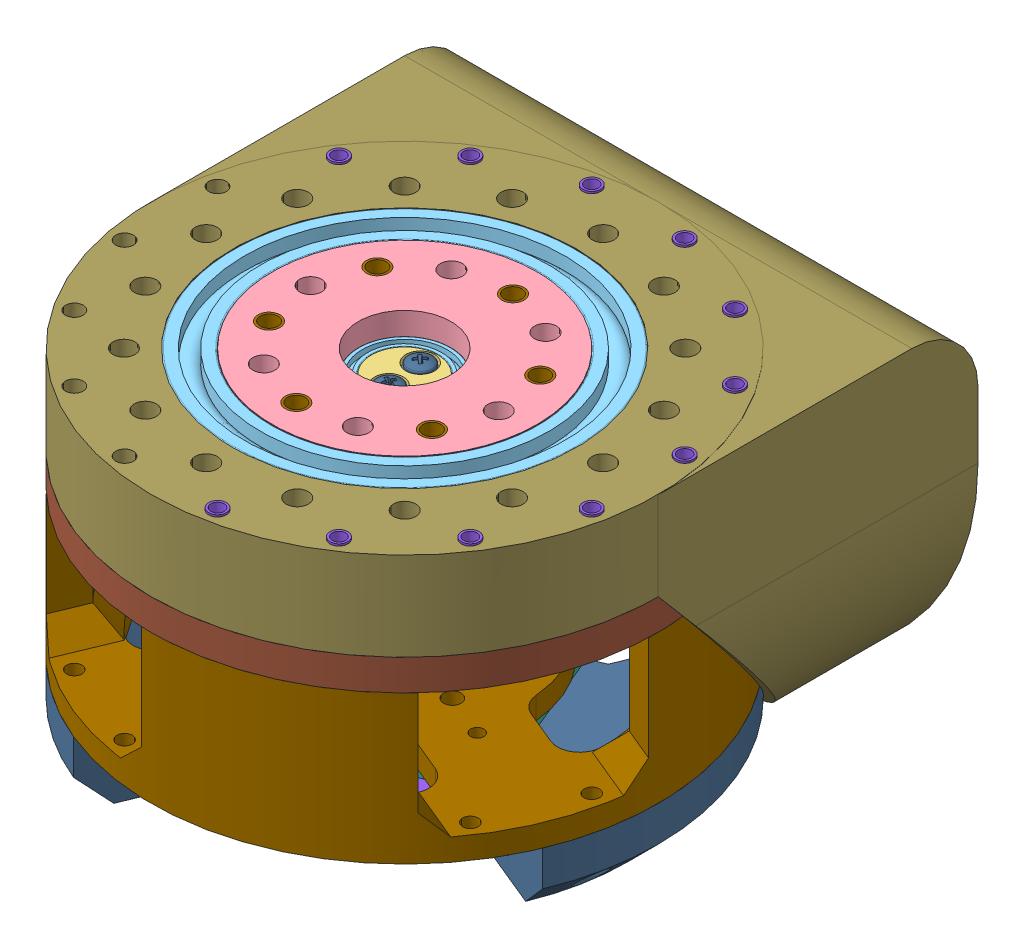
SolidWorks assembly Cycloidal_v3, configuration Default. Lengths in mm.
Overall size (150.25 88 150.25).
358 component instances, 93 part files, 116 mates.
Components (placement in the parent):
- motor-X83008S.stp-1: motor-X83008S.stp [Default] at (43.3116 89.8915 45.5734) x (0.360585 0 0.932726) z (0 -1 0) size (114.7 114.7 37.62) (hidden)
  - base.stp-1: base.stp [Default] at (42.0794 12.0269 46.7342) size (91.6 91.6 15.61)
  - stator.stp-1: stator.stp [Default] at (42.0794 12.0269 33.1342) x (0.08493 -0.996387 0) z (0 0 1) size (83 83 8)
  - coil.stp-1: coil.stp [Default] at (39.5332 41.8984 37.1342) x (0.996387 0.08493 0) z (-0.08493 0.996387 0) size (4.4 10.2 10.5)
  - coil.stp-2: coil.stp [Default] at (34.3848 41.0025 37.1342) x (0.966502 0.256661 0) z (-0.256661 0.966502 0) size (4.4 10.2 10.5)
  - coil.stp-3: coil.stp [Default] at (29.4701 39.2261 37.1342) x (0.90725 0.420593 0) z (-0.420593 0.90725 0) size (4.4 10.2 10.5)
  - coil.stp-4: coil.stp [Default] at (24.9386 36.6233 37.1342) x (0.820431 0.571745 0) z (-0.571745 0.820431 0) size (4.4 10.2 10.5)
  - coil.stp-5: coil.stp [Default] at (20.9279 33.2732 37.1342) x (0.708685 0.705525 0) z (-0.705525 0.708685 0) size (4.4 10.2 10.5)
  - coil.stp-6: coil.stp [Default] at (17.5599 29.2775 37.1342) x (0.575405 0.817869 0) z (-0.817869 0.575405 0) size (4.4 10.2 10.5)
  - coil.stp-7: coil.stp [Default] at (14.9368 24.7576 37.1342) x (0.424642 0.905361 0) z (-0.905361 0.424642 0) size (4.4 10.2 10.5)
  - coil.stp-8: coil.stp [Default] at (13.1385 19.8509 37.1342) x (0.260976 0.965345 0) z (-0.965345 0.260976 0) size (4.4 10.2 10.5)
  - coil.stp-9: coil.stp [Default] at (12.2196 14.7066 37.1342) x (0.089381 0.995998 0) z (-0.995998 0.089381 0) size (4.4 10.2 10.5)
  - coil.stp-10: coil.stp [Default] at (12.2079 9.4807 37.1342) x (-0.08493 0.996387 0) z (-0.996387 -0.08493 0) size (4.4 10.2 10.5)
  - coil.stp-11: coil.stp [Default] at (13.1039 4.3323 37.1342) x (-0.256661 0.966502 0) z (-0.966502 -0.256661 0) size (4.4 10.2 10.5)
  - coil.stp-12: coil.stp [Default] at (14.8802 -0.5824 37.1342) x (-0.420593 0.90725 0) z (-0.90725 -0.420593 0) size (4.4 10.2 10.5)
  - coil.stp-13: coil.stp [Default] at (17.483 -5.1139 37.1342) x (-0.571745 0.820431 0) z (-0.820431 -0.571745 0) size (4.4 10.2 10.5)
  - coil.stp-14: coil.stp [Default] at (20.8332 -9.1246 37.1342) x (-0.705525 0.708685 0) z (-0.708685 -0.705525 0) size (4.4 10.2 10.5)
  - coil.stp-15: coil.stp [Default] at (24.8289 -12.4926 37.1342) x (-0.817869 0.575405 0) z (-0.575405 -0.817869 0) size (4.4 10.2 10.5)
  - coil.stp-16: coil.stp [Default] at (29.3487 -15.1157 37.1342) x (-0.905361 0.424642 0) z (-0.424642 -0.905361 0) size (4.4 10.2 10.5)
  - coil.stp-17: coil.stp [Default] at (34.2554 -16.914 37.1342) x (-0.965345 0.260976 0) z (-0.260976 -0.965345 0) size (4.4 10.2 10.5)
  - coil.stp-18: coil.stp [Default] at (39.3998 -17.8329 37.1342) x (-0.995998 0.089381 0) z (-0.089381 -0.995998 0) size (4.4 10.2 10.5)
  - coil.stp-19: coil.stp [Default] at (44.6256 -17.8446 37.1342) x (-0.996387 -0.08493 0) z (0.08493 -0.996387 0) size (4.4 10.2 10.5)
  - coil.stp-20: coil.stp [Default] at (49.7741 -16.9486 37.1342) x (-0.966502 -0.256661 0) z (0.256661 -0.966502 0) size (4.4 10.2 10.5)
  - coil.stp-21: coil.stp [Default] at (54.6887 -15.1723 37.1342) x (-0.90725 -0.420593 0) z (0.420593 -0.90725 0) size (4.4 10.2 10.5)
  - coil.stp-22: coil.stp [Default] at (59.2202 -12.5695 37.1342) x (-0.820431 -0.571745 0) z (0.571745 -0.820431 0) size (4.4 10.2 10.5)
  - coil.stp-23: coil.stp [Default] at (63.2309 -9.2193 37.1342) x (-0.708685 -0.705525 0) z (0.705525 -0.708685 0) size (4.4 10.2 10.5)
  - coil.stp-24: coil.stp [Default] at (66.599 -5.2236 37.1342) x (-0.575405 -0.817869 0) z (0.817869 -0.575405 0) size (4.4 10.2 10.5)
  - coil.stp-25: coil.stp [Default] at (69.222 -0.7038 37.1342) x (-0.424642 -0.905361 0) z (0.905361 -0.424642 0) size (4.4 10.2 10.5)
  - coil.stp-26: coil.stp [Default] at (71.0203 4.2029 37.1342) x (-0.260976 -0.965345 0) z (0.965345 -0.260976 0) size (4.4 10.2 10.5)
  - coil.stp-27: coil.stp [Default] at (71.9392 9.3473 37.1342) x (-0.089381 -0.995998 0) z (0.995998 -0.089381 0) size (4.4 10.2 10.5)
  - coil.stp-28: coil.stp [Default] at (71.9509 14.5731 37.1342) x (0.08493 -0.996387 0) z (0.996387 0.08493 0) size (4.4 10.2 10.5)
  - coil.stp-29: coil.stp [Default] at (71.055 19.7216 37.1342) x (0.256661 -0.966502 0) z (0.966502 0.256661 0) size (4.4 10.2 10.5)
  - coil.stp-30: coil.stp [Default] at (69.2786 24.6362 37.1342) x (0.420593 -0.90725 0) z (0.90725 0.420593 0) size (4.4 10.2 10.5)
  - coil.stp-31: coil.stp [Default] at (66.6758 29.1677 37.1342) x (0.571745 -0.820431 0) z (0.820431 0.571745 0) size (4.4 10.2 10.5)
  - coil.stp-32: coil.stp [Default] at (63.3257 33.1785 37.1342) x (0.705525 -0.708685 0) z (0.708685 0.705525 0) size (4.4 10.2 10.5)
  - coil.stp-33: coil.stp [Default] at (59.33 36.5465 37.1342) x (0.817869 -0.575405 0) z (0.575405 0.817869 0) size (4.4 10.2 10.5)
  - coil.stp-34: coil.stp [Default] at (54.8101 39.1695 37.1342) x (0.905361 -0.424642 0) z (0.424642 0.905361 0) size (4.4 10.2 10.5)
  - coil.stp-35: coil.stp [Default] at (49.9034 40.9678 37.1342) x (0.965345 -0.260976 0) z (0.260976 0.965345 0) size (4.4 10.2 10.5)
  - coil.stp-36: coil.stp [Default] at (44.759 41.8868 37.1342) x (0.995998 -0.089381 0) z (0.089381 0.995998 0) size (4.4 10.2 10.5)
  - rotor.stp-1: rotor.stp [Default] at (42.0794 12.0269 42.1342) x (-0.293442 0.955977 0) z (0 0 -1) size (91.8 91.8 12)
  - outrunner.stp-1: outrunner.stp [Default] at (42.0794 12.0269 30.1342) x (-0.254711 0.967017 0) z (-0.967017 -0.254711 0) size (91.8 17.01 91.8)
  - screw-mount.stp-1: screw-mount.stp [Default] at (38.1314 27.0157 27.1342) x (1 0 0) z (0 0 -1) size (7 7 6.5)
  - screw-mount.stp-2: screw-mount.stp [Default] at (27.0906 8.0789 27.1342) x (1 0 0) z (0 0 -1) size (7 7 6.5)
  - screw-mount.stp-3: screw-mount.stp [Default] at (57.0682 15.9749 27.1342) x (1 0 0) z (0 0 -1) size (7 7 6.5)
  - screw-mount.stp-4: screw-mount.stp [Default] at (46.0274 -2.9618 27.1342) x (1 0 0) z (0 0 -1) size (7 7 6.5)
  - 6702ZZ-bearing-15x21x4.stp-1: 6702ZZ-bearing-15x21x4.stp [Default] at (42.0794 12.0269 43.7342) x (1 0 0) z (0 -1 0) size (21 4 21)
  - 6702ZZ-bearing-15x21x4.stp-2: 6702ZZ-bearing-15x21x4.stp [Default] at (42.0794 12.0269 35.1342) x (1 0 0) z (0 1 0) size (21 4 21)
  - shaft.stp-1: shaft.stp [Default] at (42.0794 12.0269 20.1342) size (16 16 31.6)
  - fix-screw.stp-1: fix-screw.stp [Default] at (42.0794 12.0269 51.7342) x (1 0 0) z (0 0 -1) size (19.67 18.96 12.02)
- Base_Plate-1: Base_Plate [Default] at (47.267 69.7573 89.1587) x (-0.111117 0 -0.993807) z (0.993807 0 -0.111117) size (40 7 40)
- Eccentric_Shaft-1: Eccentric_Shaft [Default] at (56.4156 70.4165 102.314) x (-0.993807 0 0.111117) z (-0.111117 0 -0.993807) size (20 15 17)
  - Eccentric_Shaft_bot-1: Eccentric_Shaft_bot [Default] at (7.6302 6.3409 14.0904) size (17 5 17)
  - Eccentric_Shaft_bot-2: Eccentric_Shaft_bot [Default] at (7.6302 11.3409 14.0904) x (-1 0 0) z (0 0 -1) size (17 5 17)
  - Eccentric_Shaft_top-1: Eccentric_Shaft_top [Default] at (7.6302 16.3409 14.0904) x (-1 0 0) z (0 0 -1) size (17 5 17)
- Output_Shaft-1: Output_Shaft [Default] at (47.267 86.8173 89.1587) x (-0.997523 0 -0.070342) z (0.070342 0 -0.997523) size (60 10 60)
- radial ball bearing_68_iso-39: radial ball bearing_68_iso [ISO 15 RBB - 1860 - 32,SI,NC,32_68] at (47.267 91.8173 89.1587) x (0 1 0) z (0.105786 0 0.994389) size (10 78 78)
- radial ball bearing_68_iso-40: radial ball bearing_68_iso [ISO 15 RBB - 1840 - 32,SI,NC,32_68] at (47.267 73.2573 89.1587) x (0 1 0) z (-0.019534 0 0.999809) size (7 52 52)
- m13_bearing-31: m13_bearing [Default] at (-10.7414 95.4081 67.0593) x (0.227678 0 0.973736) z (0.973736 0 -0.227678) size (13 16 13)
  - m6-1: m6 [Default] at (8.4921 2.5508 14.8914) size (6 16 6)
  - radial ball bearing_68_iso-1: radial ball bearing_68_iso [ISO 15 RBB - 286 - 10,SI,NC,10_68] at (8.4921 16.0508 14.8914) x (0 1 0) z (0 0 1) size (5 13 13)
  - radial ball bearing_68_iso-2: radial ball bearing_68_iso [ISO 15 RBB - 286 - 10,SI,NC,10_68] at (8.4921 11.0508 14.8914) x (0 1 0) z (0 0 1) size (5 13 13)
- m13_bearing-32: m13_bearing [Default] at (-14.1668 95.4081 84.2801) x (0.227678 0 0.973736) z (0.973736 0 -0.227678) size (13 16 13)
  - m6-1: m6 [Default] at (8.4921 2.5508 14.8914) size (6 16 6)
  - radial ball bearing_68_iso-1: radial ball bearing_68_iso [ISO 15 RBB - 286 - 10,SI,NC,10_68] at (8.4921 16.0508 14.8914) x (0 1 0) z (0 0 1) size (5 13 13)
  - radial ball bearing_68_iso-2: radial ball bearing_68_iso [ISO 15 RBB - 286 - 10,SI,NC,10_68] at (8.4921 11.0508 14.8914) x (0 1 0) z (0 0 1) size (5 13 13)
- m13_bearing-34: m13_bearing [Default] at (13.6125 95.5581 125.8547) x (0.227678 0 0.973736) z (0.973736 0 -0.227678) size (13 16 13)
  - m6-1: m6 [Default] at (8.4921 2.5508 14.8914) size (6 16 6)
  - radial ball bearing_68_iso-1: radial ball bearing_68_iso [ISO 15 RBB - 286 - 10,SI,NC,10_68] at (8.4921 16.0508 14.8914) x (0 1 0) z (0 0 1) size (5 13 13)
  - radial ball bearing_68_iso-2: radial ball bearing_68_iso [ISO 15 RBB - 286 - 10,SI,NC,10_68] at (8.4921 11.0508 14.8914) x (0 1 0) z (0 0 1) size (5 13 13)
- m13_bearing-35: m13_bearing [Default] at (-0.9866 95.4081 116.0999) x (0.227678 0 0.973736) z (0.973736 0 -0.227678) size (13 16 13)
  - m6-1: m6 [Default] at (8.4921 2.5508 14.8914) size (6 16 6)
  - radial ball bearing_68_iso-1: radial ball bearing_68_iso [ISO 15 RBB - 286 - 10,SI,NC,10_68] at (8.4921 16.0508 14.8914) x (0 1 0) z (0 0 1) size (5 13 13)
  - radial ball bearing_68_iso-2: radial ball bearing_68_iso [ISO 15 RBB - 286 - 10,SI,NC,10_68] at (8.4921 11.0508 14.8914) x (0 1 0) z (0 0 1) size (5 13 13)
- m13_bearing-36: m13_bearing [Default] at (-10.7414 95.5581 101.5009) x (0.227678 0 0.973736) z (0.973736 0 -0.227678) size (13 16 13)
  - m6-1: m6 [Default] at (8.4921 2.5508 14.8914) size (6 16 6)
  - radial ball bearing_68_iso-1: radial ball bearing_68_iso [ISO 15 RBB - 286 - 10,SI,NC,10_68] at (8.4921 16.0508 14.8914) x (0 1 0) z (0 0 1) size (5 13 13)
  - radial ball bearing_68_iso-2: radial ball bearing_68_iso [ISO 15 RBB - 286 - 10,SI,NC,10_68] at (8.4921 11.0508 14.8914) x (0 1 0) z (0 0 1) size (5 13 13)
- m13_bearing-1: m13_bearing [Default] at (-0.8801 95.4081 62.5627) x (0.736525 0 0.676411) z (0.676411 0 -0.736525) size (13 16 13)
  - m6-1: m6 [Default] at (8.4921 2.5508 14.8914) size (6 16 6)
  - radial ball bearing_68_iso-1: radial ball bearing_68_iso [ISO 15 RBB - 286 - 10,SI,NC,10_68] at (8.4921 16.0508 14.8914) x (0 1 0) z (0 0 1) size (5 13 13)
  - radial ball bearing_68_iso-2: radial ball bearing_68_iso [ISO 15 RBB - 286 - 10,SI,NC,10_68] at (8.4921 11.0508 14.8914) x (0 1 0) z (0 0 1) size (5 13 13)
- m13_bearing-2: m13_bearing [Default] at (48.6831 95.4081 124.0939) x (0.120271 0 0.992741) z (0.992741 0 -0.120271) size (13 16 13)
  - m6-1: m6 [Default] at (8.4921 2.5508 14.8914) size (6 16 6)
  - radial ball bearing_68_iso-1: radial ball bearing_68_iso [ISO 15 RBB - 286 - 10,SI,NC,10_68] at (8.4921 16.0508 14.8914) x (0 1 0) z (0 0 1) size (5 13 13)
  - radial ball bearing_68_iso-2: radial ball bearing_68_iso [ISO 15 RBB - 286 - 10,SI,NC,10_68] at (8.4921 11.0508 14.8914) x (0 1 0) z (0 0 1) size (5 13 13)
- m13_bearing-3: m13_bearing [Default] at (32.7832 95.4081 34.9886) x (-0.046141 0 0.998935) z (0.998935 0 0.046141) size (13 16 13)
  - m6-1: m6 [Default] at (8.4921 2.5508 14.8914) size (6 16 6)
  - radial ball bearing_68_iso-1: radial ball bearing_68_iso [ISO 15 RBB - 286 - 10,SI,NC,10_68] at (8.4921 16.0508 14.8914) x (0 1 0) z (0 0 1) size (5 13 13)
  - radial ball bearing_68_iso-2: radial ball bearing_68_iso [ISO 15 RBB - 286 - 10,SI,NC,10_68] at (8.4921 11.0508 14.8914) x (0 1 0) z (0 0 1) size (5 13 13)
- m13_bearing-4: m13_bearing [Default] at (77.6928 95.3081 80.133) x (-0.036208 0 0.999344) z (0.999344 0 0.036208) size (13 16 13)
  - m6-1: m6 [Default] at (8.4921 2.5508 14.8914) size (6 16 6)
  - radial ball bearing_68_iso-1: radial ball bearing_68_iso [ISO 15 RBB - 286 - 10,SI,NC,10_68] at (8.4921 16.0508 14.8914) x (0 1 0) z (0 0 1) size (5 13 13)
  - radial ball bearing_68_iso-2: radial ball bearing_68_iso [ISO 15 RBB - 286 - 10,SI,NC,10_68] at (8.4921 11.0508 14.8914) x (0 1 0) z (0 0 1) size (5 13 13)
- m13_bearing-5: m13_bearing [Default] at (73.474 95.4081 98.7828) x (0.059133 0 0.99825) z (0.99825 0 -0.059133) size (13 16 13)
  - m6-1: m6 [Default] at (8.4921 2.5508 14.8914) size (6 16 6)
  - radial ball bearing_68_iso-1: radial ball bearing_68_iso [ISO 15 RBB - 286 - 10,SI,NC,10_68] at (8.4921 16.0508 14.8914) x (0 1 0) z (0 0 1) size (5 13 13)
  - radial ball bearing_68_iso-2: radial ball bearing_68_iso [ISO 15 RBB - 286 - 10,SI,NC,10_68] at (8.4921 11.0508 14.8914) x (0 1 0) z (0 0 1) size (5 13 13)
- m13_bearing-6: m13_bearing [Default] at (12.9248 95.4081 46.7315) x (0.451561 0 0.89224) z (0.89224 0 -0.451561) size (13 16 13)
  - m6-1: m6 [Default] at (8.4921 2.5508 14.8914) size (6 16 6)
  - radial ball bearing_68_iso-1: radial ball bearing_68_iso [ISO 15 RBB - 286 - 10,SI,NC,10_68] at (8.4921 16.0508 14.8914) x (0 1 0) z (0 0 1) size (5 13 13)
  - radial ball bearing_68_iso-2: radial ball bearing_68_iso [ISO 15 RBB - 286 - 10,SI,NC,10_68] at (8.4921 11.0508 14.8914) x (0 1 0) z (0 0 1) size (5 13 13)
- m13_bearing-7: m13_bearing [Default] at (56.6452 95.4081 32.3406) x (-0.545813 0 0.837907) z (0.837907 0 0.545813) size (13 16 13)
  - m6-1: m6 [Default] at (8.4921 2.5508 14.8914) size (6 16 6)
  - radial ball bearing_68_iso-1: radial ball bearing_68_iso [ISO 15 RBB - 286 - 10,SI,NC,10_68] at (8.4921 16.0508 14.8914) x (0 1 0) z (0 0 1) size (5 13 13)
  - radial ball bearing_68_iso-2: radial ball bearing_68_iso [ISO 15 RBB - 286 - 10,SI,NC,10_68] at (8.4921 11.0508 14.8914) x (0 1 0) z (0 0 1) size (5 13 13)
- m13_bearing-8: m13_bearing [Default] at (63.0373 95.4081 51.3153) x (0.158553 0 0.98735) z (0.98735 0 -0.158553) size (13 16 13)
  - m6-1: m6 [Default] at (8.4921 2.5508 14.8914) size (6 16 6)
  - radial ball bearing_68_iso-1: radial ball bearing_68_iso [ISO 15 RBB - 286 - 10,SI,NC,10_68] at (8.4921 16.0508 14.8914) x (0 1 0) z (0 0 1) size (5 13 13)
  - radial ball bearing_68_iso-2: radial ball bearing_68_iso [ISO 15 RBB - 286 - 10,SI,NC,10_68] at (8.4921 11.0508 14.8914) x (0 1 0) z (0 0 1) size (5 13 13)
- m13_bearing-9: m13_bearing [Default] at (83.8577 95.4081 55.5358) x (-0.687134 0 0.72653) z (0.72653 0 0.687134) size (13 16 13)
  - m6-1: m6 [Default] at (8.4921 2.5508 14.8914) size (6 16 6)
  - radial ball bearing_68_iso-1: radial ball bearing_68_iso [ISO 15 RBB - 286 - 10,SI,NC,10_68] at (8.4921 16.0508 14.8914) x (0 1 0) z (0 0 1) size (5 13 13)
  - radial ball bearing_68_iso-2: radial ball bearing_68_iso [ISO 15 RBB - 286 - 10,SI,NC,10_68] at (8.4921 11.0508 14.8914) x (0 1 0) z (0 0 1) size (5 13 13)
- m13_bearing-11: m13_bearing [Default] at (30.1977 95.4081 135.7424) x (0.57351 0 0.819198) z (0.819198 0 -0.57351) size (13 16 13)
  - m6-1: m6 [Default] at (8.4921 2.5508 14.8914) size (6 16 6)
  - radial ball bearing_68_iso-1: radial ball bearing_68_iso [ISO 15 RBB - 286 - 10,SI,NC,10_68] at (8.4921 16.0508 14.8914) x (0 1 0) z (0 0 1) size (5 13 13)
  - radial ball bearing_68_iso-2: radial ball bearing_68_iso [ISO 15 RBB - 286 - 10,SI,NC,10_68] at (8.4921 11.0508 14.8914) x (0 1 0) z (0 0 1) size (5 13 13)
- m13_bearing-12: m13_bearing [Default] at (62.8861 95.4081 115.3744) x (0.184178 0 0.982893) z (0.982893 0 -0.184178) size (13 16 13)
  - m6-1: m6 [Default] at (8.4921 2.5508 14.8914) size (6 16 6)
  - radial ball bearing_68_iso-1: radial ball bearing_68_iso [ISO 15 RBB - 286 - 10,SI,NC,10_68] at (8.4921 16.0508 14.8914) x (0 1 0) z (0 0 1) size (5 13 13)
  - radial ball bearing_68_iso-2: radial ball bearing_68_iso [ISO 15 RBB - 286 - 10,SI,NC,10_68] at (8.4921 11.0508 14.8914) x (0 1 0) z (0 0 1) size (5 13 13)
- socket button head screw_iso-2: socket button head screw_iso [ISO 7380 - M4 x 12 - 12N] at (47.267 67.4573 134.1587) x (0 1 0) z (-0.724148 0 0.689645) size (14.2 7.6 7.6)
- socket button head screw_iso-3: socket button head screw_iso [ISO 7380 - M4 x 12 - 12N] at (15.4472 67.4573 57.3389) x (0 1 0) z (-0.724148 0 0.689645) size (14.2 7.6 7.6)
- socket button head screw_iso-4: socket button head screw_iso [ISO 7380 - M4 x 12 - 12N] at (30.0462 67.4573 47.5841) x (0 1 0) z (-0.724148 0 0.689645) size (14.2 7.6 7.6)
- socket button head screw_iso-5: socket button head screw_iso [ISO 7380 - M4 x 12 - 12N] at (47.267 67.4573 44.1587) x (0 1 0) z (-0.724148 0 0.689645) size (14.2 7.6 7.6)
- socket button head screw_iso-6: socket button head screw_iso [ISO 7380 - M4 x 12 - 12N] at (64.4877 67.4573 47.5841) x (0 1 0) z (-0.724148 0 0.689645) size (14.2 7.6 7.6)
- socket button head screw_iso-8: socket button head screw_iso [ISO 7380 - M4 x 12 - 12N] at (88.8416 67.4573 71.9379) x (0 1 0) z (-0.724148 0 0.689645) size (14.2 7.6 7.6)
- socket button head screw_iso-9: socket button head screw_iso [ISO 7380 - M4 x 12 - 12N] at (92.267 67.4573 89.1587) x (0 1 0) z (-0.724148 0 0.689645) size (14.2 7.6 7.6)
- socket button head screw_iso-10: socket button head screw_iso [ISO 7380 - M4 x 12 - 12N] at (88.8416 67.4573 106.3794) x (0 1 0) z (-0.724148 0 0.689645) size (14.2 7.6 7.6)
- socket button head screw_iso-11: socket button head screw_iso [ISO 7380 - M4 x 12 - 12N] at (79.0868 67.4573 120.9785) x (0 1 0) z (-0.724148 0 0.689645) size (14.2 7.6 7.6)
- M3x4x4.2_brass_insert-2: M3x4x4.2_brass_insert [Default] at (2.3676 97.2573 59.1579) x (-0.680278 0 -0.732954) z (-0.732954 0 0.680278) size (4 4 4)
- M3x4x4.2_brass_insert-3: M3x4x4.2_brass_insert [Default] at (17.2662 97.2573 44.2593) x (-0.509546 0 -0.860444) z (-0.860444 0 0.509546) size (4 4 4)
- M3x4x4.2_brass_insert-6: M3x4x4.2_brass_insert [Default] at (77.2678 97.2573 44.2593) x (-0.680278 0 -0.732954) z (-0.732954 0 0.680278) size (4 4 4)
- M3x4x4.2_brass_insert-8: M3x4x4.2_brass_insert [Default] at (100.2294 93.2573 78.6238) x (-0.970393 0 0.241533) z (-0.241533 0 -0.970393) size (4 4 4)
- M3x4x4.2_brass_insert-14: M3x4x4.2_brass_insert [Default] at (36.7321 97.2573 36.1963) x (0.509546 0 0.860444) z (0.860444 0 -0.509546) size (4 4 4)
- M3x4x4.2_brass_insert-15: M3x4x4.2_brass_insert [Default] at (57.8019 93.2573 36.1963) x (0.897191 0 -0.441644) z (0.441644 0 0.897191) size (4 4 4)
- M3x4x4.2_brass_insert-16: M3x4x4.2_brass_insert [Default] at (92.1663 97.2573 59.1579) x (-0.680278 0 -0.732954) z (-0.732954 0 0.680278) size (4 4 4)
- M3x4x4.2_brass_insert-17: M3x4x4.2_brass_insert [Default] at (100.2294 97.2573 99.6935) x (0.680278 0 0.732954) z (0.732954 0 -0.680278) size (4 4 4)
- M3x4x4.2_brass_insert-19: M3x4x4.2_brass_insert [Default] at (92.1663 97.2573 119.1595) x (0.680278 0 0.732954) z (0.732954 0 -0.680278) size (4 4 4)
- M3x4x4.2_brass_insert-20: M3x4x4.2_brass_insert [Default] at (77.2678 97.2573 134.058) x (0.680278 0 0.732954) z (0.732954 0 -0.680278) size (4 4 4)
- M3x4x4.2_brass_insert-21: M3x4x4.2_brass_insert [Default] at (57.8019 97.2573 142.1211) x (0.680278 0 0.732954) z (0.732954 0 -0.680278) size (4 4 4)
- M4x6x5.5_brass_insert-47: M4x6x5.5_brass_insert [Default] at (5.6924 92.8573 71.9379) x (0.474598 0 0.880203) z (0 1 0) size (5 5 6)
- M4x6x5.5_brass_insert-48: M4x6x5.5_brass_insert [Default] at (2.267 92.8573 89.1587) x (0.260051 0 0.965595) z (0 1 0) size (5 5 6)
- M4x6x5.5_brass_insert-49: M4x6x5.5_brass_insert [Default] at (5.6924 87.0073 106.3794) x (-0.745833 0 0.666133) z (0 -1 0) size (5 5 6)
- M4x6x5.5_brass_insert-50: M4x6x5.5_brass_insert [Default] at (15.4472 86.8573 120.9785) x (-0.745833 0 0.666133) z (0 -1 0) size (5 5 6)
- M4x6x5.5_brass_insert-51: M4x6x5.5_brass_insert [Default] at (30.0462 87.0073 130.7332) x (0.260051 0 -0.965595) z (0 -1 0) size (5 5 6)
- M4x6x5.5_brass_insert-1: M4x6x5.5_brass_insert [Default] at (37.1966 86.633 68.4805) x (-0.745833 0 0.666133) z (0 -1 0) size (5 5 6)
- M4x6x5.5_brass_insert-4: M4x6x5.5_brass_insert [Default] at (70.21 92.633 90.7765) x (0.260051 0 0.965595) z (0 1 0) size (5 5 6)
- M4x6x5.5_brass_insert-5: M4x6x5.5_brass_insert [Default] at (57.3374 92.633 109.8369) x (0.260051 0 0.965595) z (0 1 0) size (5 5 6)
- M4x6x5.5_brass_insert-6: M4x6x5.5_brass_insert [Default] at (34.3944 92.633 108.219) x (0.252509 0 0.967595) z (0 1 0) size (5 5 6)
- M4x6x5.5_brass_insert-7: M4x6x5.5_brass_insert [Default] at (24.324 92.633 87.5408) x (0.175665 0 0.98445) z (0 1 0) size (5 5 6)
- M4x6x5.5_brass_insert-8: M4x6x5.5_brass_insert [Default] at (48.8849 96.8173 66.2156) x (0.294696 0 0.955591) z (0 1 0) size (5 5 6)
- M4x6x5.5_brass_insert-9: M4x6x5.5_brass_insert [Default] at (28.2067 96.8173 76.286) x (0.260051 0 0.965595) z (0 1 0) size (5 5 6)
- M4x6x5.5_brass_insert-10: M4x6x5.5_brass_insert [Default] at (26.5888 96.8173 99.2291) x (0.009651 0 0.999953) z (0 1 0) size (5 5 6)
- M4x6x5.5_brass_insert-11: M4x6x5.5_brass_insert [Default] at (45.6491 96.8173 112.1017) x (0.260051 0 0.965595) z (0 1 0) size (5 5 6)
- M4x6x5.5_brass_insert-13: M4x6x5.5_brass_insert [Default] at (66.3273 96.8173 102.0313) x (0.260051 0 0.965595) z (0 1 0) size (5 5 6)
- M4x6x5.5_brass_insert-14: M4x6x5.5_brass_insert [Default] at (67.9452 96.8173 79.0883) x (0.260051 0 0.965595) z (0 1 0) size (5 5 6)
- M4x6x5.5_brass_insert-15: M4x6x5.5_brass_insert [Default] at (60.1396 92.633 70.0984) x (0.151918 0 0.988393) z (0 1 0) size (5 5 6)
- M4x6x5.5_brass_insert-20: M4x6x5.5_brass_insert [Default] at (64.4877 86.8573 130.7332) x (-0.745833 0 0.666133) z (0 -1 0) size (5 5 6)
- M4x6x5.5_brass_insert-21: M4x6x5.5_brass_insert [Default] at (47.267 86.8573 134.1587) x (-0.745833 0 0.666133) z (0 -1 0) size (5 5 6)
- M4x6x5.5_brass_insert-22: M4x6x5.5_brass_insert [Default] at (15.4472 86.8573 57.3389) x (0.623293 0 0.781988) z (0 -1 0) size (5 5 6)
- M4x6x5.5_brass_insert-23: M4x6x5.5_brass_insert [Default] at (30.0462 86.8573 47.5841) x (0.623293 0 0.781988) z (0 -1 0) size (5 5 6)
- M4x6x5.5_brass_insert-24: M4x6x5.5_brass_insert [Default] at (79.0868 86.8573 120.9785) x (0.541965 0 0.840401) z (0 -1 0) size (5 5 6)
- M4x6x5.5_brass_insert-25: M4x6x5.5_brass_insert [Default] at (88.8416 86.8573 106.3794) x (-0.745833 0 0.666133) z (0 -1 0) size (5 5 6)
- M4x6x5.5_brass_insert-26: M4x6x5.5_brass_insert [Default] at (92.267 86.8573 89.1587) x (-0.745833 0 0.666133) z (0 -1 0) size (5 5 6)
- M4x6x5.5_brass_insert-27: M4x6x5.5_brass_insert [Default] at (88.8416 86.8573 71.9379) x (-0.745833 0 0.666133) z (0 -1 0) size (5 5 6)
- M4x6x5.5_brass_insert-28: M4x6x5.5_brass_insert [Default] at (79.0868 92.8573 57.3389) x (0.260051 0 0.965595) z (0 1 0) size (5 5 6)
- M4x6x5.5_brass_insert-29: M4x6x5.5_brass_insert [Default] at (64.4877 86.8573 47.5841) x (-0.142939 0 0.989731) z (0 -1 0) size (5 5 6)
- M4x6x5.5_brass_insert-31: M4x6x5.5_brass_insert [Default] at (47.267 86.8573 44.1587) x (-0.220341 0 0.975423) z (0 -1 0) size (5 5 6)
- pan cross head_am-1: pan cross head_am [B18.6.7M - M3 x 0.5 x 20 Type I Cross Recessed PHMS --20N] at (46.8225 92.6573 85.1834) x (0 -1 0) z (0.748822 0 0.662771) size (22.37 5.6 5.6)
- pan cross head_am-3: pan cross head_am [B18.6.7M - M3 x 0.5 x 20 Type I Cross Recessed PHMS --20N] at (47.7115 92.6573 93.1339) x (0 -1 0) z (0.940321 0 0.340288) size (22.37 5.6 5.6)
- M3x4x4.2_brass_insert-22: M3x4x4.2_brass_insert [Default] at (46.8225 69.7573 85.1834) x (0.984578 0 -0.174944) z (0.174944 0 0.984578) size (4 4 4)
- M3x4x4.2_brass_insert-23: M3x4x4.2_brass_insert [Default] at (47.7115 69.7573 93.1339) x (0.984609 0 -0.174769) z (0.174769 0 0.984609) size (4 4 4)
- pan cross head_am-4: pan cross head_am [B18.6.7M - M3 x 0.5 x 10 Type I Cross Recessed PHMS --10N] at (48.9893 77.6573 104.5627) x (0 -1 0) z (0 0 1) size (12.37 5.6 5.6)
- pan cross head_am-5: pan cross head_am [B18.6.7M - M3 x 0.5 x 10 Type I Cross Recessed PHMS --10N] at (45.5447 77.6573 73.7547) x (0 -1 0) z (0 0 1) size (12.37 5.6 5.6)
- pan cross head_am-6: pan cross head_am [B18.6.7M - M3 x 0.5 x 10 Type I Cross Recessed PHMS --10N] at (62.671 77.6573 87.4364) x (0 -1 0) z (0 0 1) size (12.37 5.6 5.6)
- pan cross head_am-7: pan cross head_am [B18.6.7M - M3 x 0.5 x 10 Type I Cross Recessed PHMS --10N] at (31.863 77.6573 90.881) x (0 -1 0) z (0 0 1) size (12.37 5.6 5.6)
- radial ball bearing_68_iso-44: radial ball bearing_68_iso [ISO 15 RBB - 1715 - 26,SI,NC,26_68] at (45.7763 84.7573 89.3253) x (0 1 0) z (-0.714953 0 -0.699173) size (4 21 21)
- radial ball bearing_68_iso-45: radial ball bearing_68_iso [ISO 15 RBB - 1715 - 26,SI,NC,26_68] at (47.267 89.7573 89.1587) x (0 1 0) z (0.999483 0 -0.032163) size (4 21 21)
- radial ball bearing_68_iso-46: radial ball bearing_68_iso [ISO 15 RBB - 1715 - 26,SI,NC,26_68] at (48.7577 79.7573 88.992) x (0 1 0) z (0.000177 0 1) size (4 21 21)
- socket button head screw_iso-37: socket button head screw_iso [ISO 7380 - M4 x 12 - 12N] at (79.0868 67.4573 57.3389) x (0 1 0) z (-0.709975 0 0.704227) size (14.2 7.6 7.6)
- socket button head screw_iso-38: socket button head screw_iso [ISO 7380 - M4 x 12 - 12N] at (64.4877 67.4573 130.7332) x (0 1 0) z (-0.724148 0 0.689645) size (14.2 7.6 7.6)
- foc-motor-controller.step-1: foc-motor-controller.step [Default] at (47.267 33.7573 89.1587) x (-0.382683 0 -0.92388) z (0 -1 0) size (57.23 50 8.13)
  - RTA0040B.step-1: RTA0040B.step [Default] at (12.5014 -1.6986 1.595) x (-0.707107 -0.707107 0) z (0 0 1) size (6 6 1)
    - FRAME.step-1: FRAME.step [Default] x (1 0 0) z (0 -1 0) size (6 0.2 6)
      - SOLID.step-1: SOLID.step [Default] at origin size (0.4 0.2 0.22)
      - SOLID-0.step-1: SOLID-0.step [Default] at origin size (0.4 0.2 0.22)
      - SOLID-1.step-1: SOLID-1.step [Default] at origin size (0.4 0.2 0.22)
      - SOLID-2.step-1: SOLID-2.step [Default] at origin size (0.4 0.2 0.22)
      - SOLID-3.step-1: SOLID-3.step [Default] at origin size (0.4 0.2 0.22)
      - SOLID-4.step-1: SOLID-4.step [Default] at origin size (0.4 0.2 0.22)
      - SOLID-5.step-1: SOLID-5.step [Default] at origin size (0.4 0.2 0.22)
      - SOLID-6.step-1: SOLID-6.step [Default] at origin size (0.4 0.2 0.22)
      - SOLID-7.step-1: SOLID-7.step [Default] at origin size (0.4 0.2 0.22)
      - SOLID-8.step-1: SOLID-8.step [Default] at origin size (0.4 0.2 0.22)
      - SOLID-9.step-1: SOLID-9.step [Default] at origin size (0.22 0.2 0.4)
      - SOLID-10.step-1: SOLID-10.step [Default] at origin size (0.22 0.2 0.4)
      - SOLID-11.step-1: SOLID-11.step [Default] at origin size (0.22 0.2 0.4)
      - SOLID-12.step-1: SOLID-12.step [Default] at origin size (0.22 0.2 0.4)
      - SOLID-13.step-1: SOLID-13.step [Default] at origin size (0.22 0.2 0.4)
      - SOLID-14.step-1: SOLID-14.step [Default] at origin size (0.22 0.2 0.4)
      - SOLID-15.step-1: SOLID-15.step [Default] at origin size (0.22 0.2 0.4)
      - SOLID-16.step-1: SOLID-16.step [Default] at origin size (0.22 0.2 0.4)
      - SOLID-17.step-1: SOLID-17.step [Default] at origin size (4.15 0.2 4.15)
      - SOLID-18.step-1: SOLID-18.step [Default] at origin size (0.28 0.1 0.28)
      - SOLID-19.step-1: SOLID-19.step [Default] at origin size (0.28 0.1 0.28)
      - SOLID-20.step-1: SOLID-20.step [Default] at origin size (0.28 0.1 0.28)
      - SOLID-21.step-1: SOLID-21.step [Default] at origin size (0.28 0.1 0.28)
      - SOLID-22.step-1: SOLID-22.step [Default] at origin size (0.4 0.2 0.22)
      - SOLID-23.step-1: SOLID-23.step [Default] at origin size (0.4 0.2 0.22)
      - SOLID-24.step-1: SOLID-24.step [Default] at origin size (0.4 0.2 0.22)
      - SOLID-25.step-1: SOLID-25.step [Default] at origin size (0.4 0.2 0.22)
      - SOLID-26.step-1: SOLID-26.step [Default] at origin size (0.4 0.2 0.22)
      - SOLID-27.step-1: SOLID-27.step [Default] at origin size (0.4 0.2 0.22)
      - SOLID-28.step-1: SOLID-28.step [Default] at origin size (0.4 0.2 0.22)
      - SOLID-29.step-1: SOLID-29.step [Default] at origin size (0.4 0.2 0.22)
      - SOLID-30.step-1: SOLID-30.step [Default] at origin size (0.4 0.2 0.22)
      - SOLID-31.step-1: SOLID-31.step [Default] at origin size (0.4 0.2 0.22)
      - SOLID-32.step-1: SOLID-32.step [Default] at origin size (0.22 0.2 0.4)
      - SOLID-33.step-1: SOLID-33.step [Default] at origin size (0.22 0.2 0.4)
      - SOLID-34.step-1: SOLID-34.step [Default] at origin size (0.22 0.2 0.4)
      - SOLID-35.step-1: SOLID-35.step [Default] at origin size (0.22 0.2 0.4)
      - SOLID-36.step-1: SOLID-36.step [Default] at origin size (0.22 0.2 0.4)
      - SOLID-37.step-1: SOLID-37.step [Default] at origin size (0.22 0.2 0.4)
      - SOLID-38.step-1: SOLID-38.step [Default] at origin size (0.22 0.2 0.4)
      - SOLID-39.step-1: SOLID-39.step [Default] at origin size (0.22 0.2 0.4)
      - SOLID-40.step-1: SOLID-40.step [Default] at origin size (0.22 0.2 0.4)
      - SOLID-41.step-1: SOLID-41.step [Default] at origin size (0.22 0.2 0.4)
      - SOLID-42.step-1: SOLID-42.step [Default] at origin size (0.22 0.2 0.4)
      - SOLID-43.step-1: SOLID-43.step [Default] at origin size (0.22 0.2 0.4)
    - BODY.step-1: BODY.step [Default] at (0 0 0.025) x (1 0 0) z (0 -1 0) size (6 0.97 6)
  - Resonator_SMD_Murata_CSTxExxV-3Pin_3.0x1.1mm.step-1: Resonator_SMD_Murata_CSTxExxV-3Pin_3.0x1.1mm.step [Default] at (1.8 -7 1.595) x (0 1 0) z (0 0 1) size (3.2 1.35 0.9)
  - C_0603_1608Metric.step-1: C_0603_1608Metric.step [Default] at (6.2 -16.8 1.595) x (0 -1 0) z (0 0 1) size (1.6 0.8 0.8)
  - R_0603_1608Metric.step-1: R_0603_1608Metric.step [Default] at (11.8 -7.375 1.595) x (0 1 0) z (0 0 1) size (1.6 0.8 0.45)
  - R_0603_1608Metric.step-2: R_0603_1608Metric.step [Default] at (13.8 -16.8 1.595) x (0 1 0) z (0 0 1) size (1.6 0.8 0.45)
  - R_0603_1608Metric.step-3: R_0603_1608Metric.step [Default] at (18.1 -5.36 1.595) size (1.6 0.8 0.45)
  - C_0603_1608Metric.step-2: C_0603_1608Metric.step [Default] at (2.6 -0.5 1.595) x (0 -1 0) z (0 0 1) size (1.6 0.8 0.8)
  - R_0603_1608Metric.step-4: R_0603_1608Metric.step [Default] at (14.6 -11.3 1.595) x (0 1 0) z (0 0 1) size (1.6 0.8 0.45)
  - L_APV_ANR4020.step-1: L_APV_ANR4020.step [Default] at (22.3 -13.7 1.595) x (0 -1 0) z (0 0 1) size (4.02 4 2)
  - C_0603_1608Metric.step-3: C_0603_1608Metric.step [Default] at (0.3 -12.6 1.595) x (-1 0 0) z (0 0 1) size (1.6 0.8 0.8)
  - C_1206_3216Metric.step-1: C_1206_3216Metric.step [Default] at (15.7 11 1.595) x (0 1 0) z (0 0 1) size (3.2 1.6 1.6)
  - C_0603_1608Metric.step-4: C_0603_1608Metric.step [Default] at (0.3 -9.6 1.595) size (1.6 0.8 0.8)
  - R_0603_1608Metric.step-5: R_0603_1608Metric.step [Default] at (12.3 -16.8 1.595) x (0 1 0) z (0 0 1) size (1.6 0.8 0.45)
  - C_0603_1608Metric.step-5: C_0603_1608Metric.step [Default] at (-0.3 -16.6 1.595) x (0 1 0) z (0 0 1) size (1.6 0.8 0.8)
  - R_0603_1608Metric.step-6: R_0603_1608Metric.step [Default] at (10.9 4.1 1.595) size (1.6 0.8 0.45)
  - C_1206_3216Metric.step-2: C_1206_3216Metric.step [Default] at (6.3 11 1.595) x (0 1 0) z (0 0 1) size (3.2 1.6 1.6)
  - XT30PW_2_2_-M.G.B.step-1: XT30PW_2_2_-M.G.B.step [Default] at (-20.5 9.5 1.595) x (0 -1 0) z (-1 0 0) size (15.5 7.1 12.53)
  - R_0603_1608Metric.step-7: R_0603_1608Metric.step [Default] at (0.3 -11.1 1.595) size (1.6 0.8 0.45)
  - C_0603_1608Metric.step-6: C_0603_1608Metric.step [Default] at (19 -0.4 1.595) x (-0.707107 -0.707107 0) z (0 0 1) size (1.6 0.8 0.8)
  - C_1206_3216Metric.step-3: C_1206_3216Metric.step [Default] at (13.3 11 1.595) x (0 1 0) z (0 0 1) size (3.2 1.6 1.6)
  - R_0603_1608Metric.step-8: R_0603_1608Metric.step [Default] at (10.2 -7.375 1.595) x (0 -1 0) z (0 0 1) size (1.6 0.8 0.45)
  - JST_GH_SM08B-GHS-TB_1x08-1MP_P1.25mm_Horizontal.step-1: JST_GH_SM08B-GHS-TB_1x08-1MP_P1.25mm_Horizontal.step [Default] at (10 -22 1.595) size (13.25 4.95 4.25)
  - C_1206_3216Metric.step-4: C_1206_3216Metric.step [Default] at (-12.3 11 1.595) x (0 1 0) z (0 0 1) size (3.2 1.6 1.6)
  - JST_GH_SM06B-GHS-TB_1x06-1MP_P1.25mm_Horizontal.step-1: JST_GH_SM06B-GHS-TB_1x06-1MP_P1.25mm_Horizontal.step [Default] at (-4.3 -22 1.595) size (10.75 4.95 4.25)
  - C_0603_1608Metric.step-7: C_0603_1608Metric.step [Default] at (7.3 -4.5 1.595) x (-1 0 0) z (0 0 1) size (1.6 0.8 0.8)
  - R_0603_1608Metric.step-9: R_0603_1608Metric.step [Default] at (18.1 -3.86 1.595) x (-1 0 0) z (0 0 1) size (1.6 0.8 0.45)
  - C_1206_3216Metric.step-5: C_1206_3216Metric.step [Default] at (22.6794 -1.2206 1.595) x (0.707107 -0.707107 0) z (0 0 1) size (3.2 1.6 1.6)
  - R_Array_Convex_4x0402.step-1: R_Array_Convex_4x0402.step [Default] at (6.8 -2.5 1.595) size (1 2 0.35)
  - R_0603_1608Metric.step-10: R_0603_1608Metric.step [Default] at (7.7 -16.8 1.595) x (0 -1 0) z (0 0 1) size (1.6 0.8 0.45)
  - C_1206_3216Metric.step-6: C_1206_3216Metric.step [Default] at (8.7 11 1.595) x (0 1 0) z (0 0 1) size (3.2 1.6 1.6)
  - C_0603_1608Metric.step-8: C_0603_1608Metric.step [Default] at (16.1 -11.3 1.595) x (0 1 0) z (0 0 1) size (1.6 0.8 0.8)
  - SOT-23-5.step-1: SOT-23-5.step [Default] at (-3.1 -16.6 1.595) x (-1 0 0) z (0 0 1) size (2.8 2.9 1.55)
  - C_0603_1608Metric.step-9: C_0603_1608Metric.step [Default] at (17.8 -13.6 1.595) size (1.6 0.8 0.8)
  - R_0603_1608Metric.step-11: R_0603_1608Metric.step [Default] at (-11.5 -20.3875 1.595) x (0 -1 0) z (0 0 1) size (1.6 0.8 0.45)
  - C_0603_1608Metric.step-10: C_0603_1608Metric.step [Default] at (-12.4 2.3 1.595) x (0 1 0) z (0 0 1) size (1.6 0.8 0.8)
  - C_1206_3216Metric.step-7: C_1206_3216Metric.step [Default] at (18 11 1.595) x (0 1 0) z (0 0 1) size (3.2 1.6 1.6)
  - R_0603_1608Metric.step-12: R_0603_1608Metric.step [Default] at (-10.8105 -14.9971 1.595) x (-1 0 0) z (0 0 1) size (1.6 0.8 0.45)
  - C_0603_1608Metric.step-11: C_0603_1608Metric.step [Default] at (-13.8 -9.4 1.595) x (-1 0 0) z (0 0 1) size (1.6 0.8 0.8)
  - R_0603_1608Metric.step-13: R_0603_1608Metric.step [Default] at (-23.15 -14.5 1.595) x (-1 0 0) z (0 0 1) size (1.6 0.8 0.45)
  - C_0603_1608Metric.step-12: C_0603_1608Metric.step [Default] at (1.1 -0.2 1.595) x (0 1 0) z (0 0 1) size (1.6 0.8 0.8)
  - D_0805_2012Metric.step-1: D_0805_2012Metric.step [Default] at (22.9 -9.6 1.595) x (0 1 0) z (0 0 1) size (2 1.27 0.8)
  - C_0603_1608Metric.step-13: C_0603_1608Metric.step [Default] at (-7.8 3.775 1.595) x (0 -1 0) z (0 0 1) size (1.6 0.8 0.8)
  - R_0603_1608Metric.step-14: R_0603_1608Metric.step [Default] at (-6.4 -12.825 1.595) x (0 1 0) z (0 0 1) size (1.6 0.8 0.45)
  - L_0603_1608Metric.step-1: L_0603_1608Metric.step [Default] at (-10.1 3 1.595) size (1.6 0.8 0.8)
  - C_0603_1608Metric.step-14: C_0603_1608Metric.step [Default] at (17.9 0.7 1.595) x (-0.707107 -0.707107 0) z (0 0 1) size (1.6 0.8 0.8)
  - HVSSOP-10.step-1: HVSSOP-10.step [Default] at (18.6 -9.6 1.595) x (0 -1 0) z (-1 0 0) size (4.9 1.1 3)
  - C_0603_1608Metric.step-15: C_0603_1608Metric.step [Default] at (7.9 4.1 1.595) x (-1 0 0) z (0 0 1) size (1.6 0.8 0.8)
  - C_0603_1608Metric.step-16: C_0603_1608Metric.step [Default] at (21.1 -9.6 1.595) x (0 -1 0) z (0 0 1) size (1.6 0.8 0.8)
  - R_0603_1608Metric.step-15: R_0603_1608Metric.step [Default] at (-10.8105 -11.9971 1.595) x (-1 0 0) z (0 0 1) size (1.6 0.8 0.45)
  - R_0603_1608Metric.step-16: R_0603_1608Metric.step [Default] at (-18.2 -17.4 1.595) size (1.6 0.8 0.45)
  - C_1206_3216Metric.step-8: C_1206_3216Metric.step [Default] at (-3 11 1.595) x (0 1 0) z (0 0 1) size (3.2 1.6 1.6)
  - R_0603_1608Metric.step-17: R_0603_1608Metric.step [Default] at (-16.9 -20.4 1.595) x (0 -1 0) z (0 0 1) size (1.6 0.8 0.45)
  - R_0603_1608Metric.step-18: R_0603_1608Metric.step [Default] at (-13.3 -20.3875 1.595) x (0 -1 0) z (0 0 1) size (1.6 0.8 0.45)
  - R_0603_1608Metric.step-19: R_0603_1608Metric.step [Default] at (-15.1 -20.3875 1.595) x (0 -1 0) z (0 0 1) size (1.6 0.8 0.45)
  - C_0603_1608Metric.step-17: C_0603_1608Metric.step [Default] at (15.5 -14.4 1.595) x (0 -1 0) z (0 0 1) size (1.6 0.8 0.8)
  - LED_0603_1608Metric.step-1: LED_0603_1608Metric.step [Default] at (-11.5 -23.3875 1.595) x (0 1 0) z (0 0 1) size (1.6 0.8 1.1)
  - C_0805_2012Metric.step-1: C_0805_2012Metric.step [Default] at (19.95 -17 1.595) size (2 1.25 1.25)
  - D_SMB.step-1: D_SMB.step [Default] at (-16.5 11.208 1.595) x (0 -1 0) z (0 0 1) size (5.3 3.55 2.15)
  - C_1206_3216Metric.step-9: C_1206_3216Metric.step [Default] at (-5.3 11 1.595) x (0 1 0) z (0 0 1) size (3.2 1.6 1.6)
  - XT30PW_2_2_-M.G.B.step-2: XT30PW_2_2_-M.G.B.step [Default] at (-20.5 -6.5 1.595) x (0 -1 0) z (-1 0 0) size (15.5 7.1 12.53)
  - C_1206_3216Metric.step-10: C_1206_3216Metric.step [Default] at (1.7 11 1.595) x (0 1 0) z (0 0 1) size (3.2 1.6 1.6)
  - C_1206_3216Metric.step-11: C_1206_3216Metric.step [Default] at (11 11 1.595) x (0 1 0) z (0 0 1) size (3.2 1.6 1.6)
  - C_0603_1608Metric.step-18: C_0603_1608Metric.step [Default] at (-6.3 3.775 1.595) x (0 -1 0) z (0 0 1) size (1.6 0.8 0.8)
  - C_0603_1608Metric.step-19: C_0603_1608Metric.step [Default] at (16.8686 1.7314 1.595) x (0.707107 0.707107 0) z (0 0 1) size (1.6 0.8 0.8)
  - C_0603_1608Metric.step-20: C_0603_1608Metric.step [Default] at (-15.0105 -11.1 1.595) size (1.6 0.8 0.8)
  - C_1206_3216Metric.step-12: C_1206_3216Metric.step [Default] at (-7.7 11 1.595) x (0 1 0) z (0 0 1) size (3.2 1.6 1.6)
  - C_0603_1608Metric.step-21: C_0603_1608Metric.step [Default] at (-18.2 -15.8 1.595) size (1.6 0.8 0.8)
  - C_0603_1608Metric.step-22: C_0603_1608Metric.step [Default] at (-2.1 -11.3 1.595) x (0 -1 0) z (0 0 1) size (1.6 0.8 0.8)
  - C_0603_1608Metric.step-23: C_0603_1608Metric.step [Default] at (-10.8105 -13.4971 1.595) size (1.6 0.8 0.8)
  - C_1206_3216Metric.step-13: C_1206_3216Metric.step [Default] at (4 11 1.595) x (0 1 0) z (0 0 1) size (3.2 1.6 1.6)
  - R_0603_1608Metric.step-20: R_0603_1608Metric.step [Default] at (16 -17.8 1.595) x (0 1 0) z (0 0 1) size (1.6 0.8 0.45)
  - Texas_S-PVSON-N8.step-1: Texas_S-PVSON-N8.step [Default] at (-14.4105 -13.7 1.595) x (-1 0 0) z (0 0 1) size (3 2.98 0.92)
  - C_1206_3216Metric.step-14: C_1206_3216Metric.step [Default] at (21 -2.9 1.595) x (0.707107 -0.707107 0) z (0 0 1) size (3.2 1.6 1.6)
  - C_0603_1608Metric.step-24: C_0603_1608Metric.step [Default] at (-5.9 -16.6 1.595) x (0 1 0) z (0 0 1) size (1.6 0.8 0.8)
  - C_0603_1608Metric.step-25: C_0603_1608Metric.step [Default] at (-3.1 -14.1 1.595) size (1.6 0.8 0.8)
  - R_0603_1608Metric.step-21: R_0603_1608Metric.step [Default] at (7.2 -7.375 1.595) x (0 -1 0) z (0 0 1) size (1.6 0.8 0.45)
  - C_1206_3216Metric.step-15: C_1206_3216Metric.step [Default] at (-0.7 11 1.595) x (0 1 0) z (0 0 1) size (3.2 1.6 1.6)
  - LQFP-64_10x10mm_P0.5mm.step-1: LQFP-64_10x10mm_P0.5mm.step [Default] at (-7 -4.5 1.595) x (-1 0 0) z (0 0 1) size (12 12 1.5)
  - C_0805_2012Metric.step-2: C_0805_2012Metric.step [Default] at (23.35 -17 1.595) x (-1 0 0) z (0 0 1) size (2 1.25 1.25)
  - C_0603_1608Metric.step-26: C_0603_1608Metric.step [Default] at (10.8 -16.8 1.595) x (0 -1 0) z (0 0 1) size (1.6 0.8 0.8)
  - R_0603_1608Metric.step-22: R_0603_1608Metric.step [Default] at (17.5 -17.8 1.595) x (0 -1 0) z (0 0 1) size (1.6 0.8 0.45)
  - C_1206_3216Metric.step-16: C_1206_3216Metric.step [Default] at (20.3 11 1.595) x (0 1 0) z (0 0 1) size (3.2 1.6 1.6)
  - R_0603_1608Metric.step-23: R_0603_1608Metric.step [Default] at (9.2 -16.8 1.595) x (0 -1 0) z (0 0 1) size (1.6 0.8 0.45)
  - C_1206_3216Metric.step-17: C_1206_3216Metric.step [Default] at (-10 11 1.595) x (0 1 0) z (0 0 1) size (3.2 1.6 1.6)
  - R_0603_1608Metric.step-24: R_0603_1608Metric.step [Default] at (17.8 -15.2 1.595) size (1.6 0.8 0.45)
